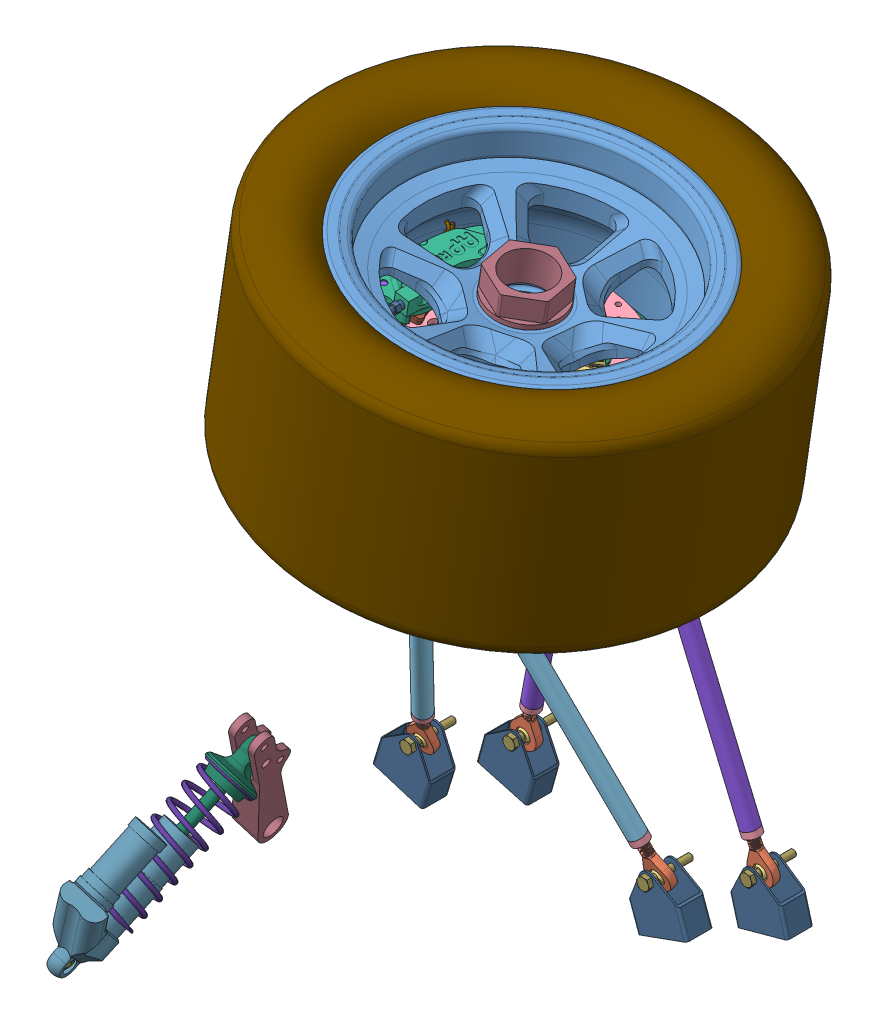
SolidWorks assembly WT-A0100-XA-Unsprung Front Axle Assembly, configuration Default. Lengths in mm.
Overall size (453.69 633.67 594.25).
81 component instances, 33 part files, 11 mates.
Components (placement in the parent):
- SP-A0200-AA-Upper Axle Assembly-1: SP-A0200-AA-Upper Axle Assembly [Default] at (-0.0001 -38.1 0) size (303.98 482.71 550.62)
  - Upper A-Arm^SP-A0200-AA-Upper Axle Assembly-1: Upper A-Arm^SP-A0200-AA-Upper Axle Assembly [Default] at (0 340.1778 -103.3743) x (1 0 0) z (0 -0.807933 0.589274) size (261.83 325.63 241.57) (virtual)
    - SP-Upper Apex Front-1: SP-Upper Apex Front [Default] at (789.6198 444.1063 49.8797) x (0.9592 -0.229397 0.165266) z (0 0.584537 0.811367) size (51.11 64.07 9.53)
    - MirrorFS-MALE ROD END UNF-3A, 0.3125x24-0.25D (XAM-4)1-1: MirrorFS-MALE ROD END UNF-3A, 0.3125x24-0.25D (XAM-4)1 [Default] at (912.4748 153.0246 259.5852) x (-0.946047 -0.262907 0.189408) z (0.32403 -0.767591 0.553) size (26.22 11.39 62.85)
      - MirrorBody^MirrorFS-MALE ROD END UNF-3A, 0.3125x24-0.25D (XAM-4)1-1: MirrorBody^MirrorFS-MALE ROD END UNF-3A, 0.3125x24-0.25D (XAM-4)1 [Default] at origin size (26.22 9.76 62.85) (virtual)
      - MirrorBall^MirrorFS-MALE ROD END UNF-3A, 0.3125x24-0.25D (XAM-4)1-1: MirrorBall^MirrorFS-MALE ROD END UNF-3A, 0.3125x24-0.25D (XAM-4)1 [Default] x (0.874091 -0.054164 -0.482733) z (-0.485762 -0.097546 -0.868631) size (12.7 9.53 12.7) (virtual)
    - MirrorFS-MALE ROD END UNF-3A, 0.3125x24-0.25D (XAM-4)1-2: MirrorFS-MALE ROD END UNF-3A, 0.3125x24-0.25D (XAM-4)1 [Default] at (683.8748 153.0246 259.5852) x (0.9592 -0.229397 0.165266) z (-0.28273 -0.778263 0.560688) size (26.22 11.39 62.85)
      - MirrorBody^MirrorFS-MALE ROD END UNF-3A, 0.3125x24-0.25D (XAM-4)1-1: MirrorBody^MirrorFS-MALE ROD END UNF-3A, 0.3125x24-0.25D (XAM-4)1 [Default] at origin size (26.22 9.76 62.85) (virtual)
      - MirrorBall^MirrorFS-MALE ROD END UNF-3A, 0.3125x24-0.25D (XAM-4)1-1: MirrorBall^MirrorFS-MALE ROD END UNF-3A, 0.3125x24-0.25D (XAM-4)1 [Default] x (0.874091 -0.054164 -0.482733) z (-0.485762 -0.097546 -0.868631) size (12.7 9.53 12.7) (virtual)
    - SP-10003-AB-Threaded Insert-1: SP-10003-AB-Threaded Insert [A-Arm] at (696.8946 188.8638 233.7654) x (-0.9592 0.229397 -0.165266) z (-0.28273 -0.778263 0.560688) size (15.88 15.88 15.88)
    - SP-10003-AB-Threaded Insert-2: SP-10003-AB-Threaded Insert [A-Arm] at (897.5532 188.3723 234.1194) x (0 0.584537 0.811367) z (0.32403 -0.767591 0.553) size (15.88 15.88 15.88)
    - SP-Upper A-Arm Tube-1: SP-Upper A-Arm Tube [Default] at (736.7473 298.5655 154.7324) x (0 -0.584537 -0.811367) z (0.9592 -0.229397 0.165266) size (15.88 313.5 15.88)
    - SP-Upper A-Arm Tube-2: SP-Upper A-Arm Tube [Default] at (851.8788 296.5698 156.1702) x (0 -0.584537 -0.811367) z (0.946047 0.262907 -0.189408) size (15.88 313.5 15.88)
    - FS-HIGH MISALIGN SPHERICAL BEARING, 0.375-0.906D (3072-6G)-1: FS-HIGH MISALIGN SPHERICAL BEARING, 0.375-0.906D (3072-6G) [Default] at (789.6198 444.1063 49.8797) x (-0.28273 -0.778263 0.560688) z (-0.9592 0.229397 -0.165266) size (26.46 21.71 26.13)
      - Race^FS-HIGH MISALIGN SPHERICAL BEARING, 0.375-0.906D (3072-6G)-1: Race^FS-HIGH MISALIGN SPHERICAL BEARING, 0.375-0.906D (3072-6G) [Default] at origin size (23.01 8.76 23.01) (virtual)
      - Ball^FS-HIGH MISALIGN SPHERICAL BEARING, 0.375-0.906D (3072-6G)-1: Ball^FS-HIGH MISALIGN SPHERICAL BEARING, 0.375-0.906D (3072-6G) [Default] x (0.359576 -0.008176 0.93308) z (-0.932238 -0.046516 0.358844) size (19.84 20.65 19.84) (virtual)
  - Lower A-Arm^SP-A0200-AA-Upper Axle Assembly-1: Lower A-Arm^SP-A0200-AA-Upper Axle Assembly [Default] at (0 -0.114 0.1797) x (1 0 0) z (0 0.000904 1) size (260.91 451.43 64.04) (virtual)
    - SP-Front Lower A-Arm Tube-2: SP-Front Lower A-Arm Tube [Default] at (852.4436 392.8879 96.9776) x (0.263467 -0.959286 -0.101763) z (0 -0.105491 0.99442) size (374.92 15.88 15.88)
    - MirrorFS-MALE ROD END UNF-3A, 0.3125x24-0.25D (XAM-4)1-1: MirrorFS-MALE ROD END UNF-3A, 0.3125x24-0.25D (XAM-4)1 [Default] at (912.4748 174.3139 73.7908) x (0.964668 0.261997 0.027793) z (0.263467 -0.959286 -0.101763) size (26.22 11.39 62.85)
      - MirrorBody^MirrorFS-MALE ROD END UNF-3A, 0.3125x24-0.25D (XAM-4)1-1: MirrorBody^MirrorFS-MALE ROD END UNF-3A, 0.3125x24-0.25D (XAM-4)1 [Default] at origin size (26.22 9.76 62.85) (virtual)
      - MirrorBall^MirrorFS-MALE ROD END UNF-3A, 0.3125x24-0.25D (XAM-4)1-1: MirrorBall^MirrorFS-MALE ROD END UNF-3A, 0.3125x24-0.25D (XAM-4)1 [Default] x (0.874091 -0.054164 -0.482733) z (-0.485762 -0.097546 -0.868631) size (12.7 9.53 12.7) (virtual)
    - MirrorFS-MALE ROD END UNF-3A, 0.3125x24-0.25D (XAM-4)1-2: MirrorFS-MALE ROD END UNF-3A, 0.3125x24-0.25D (XAM-4)1 [Default] at (683.8748 174.3139 73.7908) x (0.964668 -0.261997 -0.027793) z (-0.263467 -0.959286 -0.101763) size (26.22 11.39 62.85)
      - MirrorBody^MirrorFS-MALE ROD END UNF-3A, 0.3125x24-0.25D (XAM-4)1-1: MirrorBody^MirrorFS-MALE ROD END UNF-3A, 0.3125x24-0.25D (XAM-4)1 [Default] at origin size (26.22 9.76 62.85) (virtual)
      - MirrorBall^MirrorFS-MALE ROD END UNF-3A, 0.3125x24-0.25D (XAM-4)1-1: MirrorBall^MirrorFS-MALE ROD END UNF-3A, 0.3125x24-0.25D (XAM-4)1 [Default] x (0.874091 -0.054164 -0.482733) z (-0.485762 -0.097546 -0.868631) size (12.7 9.53 12.7) (virtual)
    - SP-Lower Apex Front-1: SP-Lower Apex Front [Default] at (798.1748 590.481 117.9388) x (0.964668 -0.261997 -0.027793) z (0 -0.105491 0.99442) size (48.15 64.07 9.53)
    - SP-10003-AB-Threaded Insert-1: SP-10003-AB-Threaded Insert [A-Arm] at (900.7637 216.9541 78.3142) x (0.964668 0.261997 0.027793) z (0.263467 -0.959286 -0.101763) size (15.88 15.88 15.88)
    - SP-10003-AB-Threaded Insert-2: SP-10003-AB-Threaded Insert [A-Arm] at (695.5859 216.9541 78.3142) x (0.964668 -0.261997 -0.027793) z (-0.263467 -0.959286 -0.101763) size (15.88 15.88 15.88)
    - FS-HIGH MISALIGN SPHERICAL BEARING, 0.375-0.906D (3072-6G)-1: FS-HIGH MISALIGN SPHERICAL BEARING, 0.375-0.906D (3072-6G) [Default] at (798.1748 590.481 117.9388) x (0.263467 0.959286 0.101763) z (-0.964668 0.261997 0.027793) size (26.46 21.71 26.13)
      - Race^FS-HIGH MISALIGN SPHERICAL BEARING, 0.375-0.906D (3072-6G)-1: Race^FS-HIGH MISALIGN SPHERICAL BEARING, 0.375-0.906D (3072-6G) [Default] at origin size (23.01 8.76 23.01) (virtual)
      - Ball^FS-HIGH MISALIGN SPHERICAL BEARING, 0.375-0.906D (3072-6G)-1: Ball^FS-HIGH MISALIGN SPHERICAL BEARING, 0.375-0.906D (3072-6G) [Default] x (0.359576 -0.008176 0.93308) z (-0.932238 -0.046516 0.358844) size (19.84 20.65 19.84) (virtual)
    - SP-Front Lower A-Arm Tube-3: SP-Front Lower A-Arm Tube [Default] at (743.906 392.8879 96.9776) x (-0.263467 -0.959286 -0.101763) z (0 -0.105491 0.99442) size (374.92 15.88 15.88)
  - SP-C30066-AA-A-Arm Tab Box-2: SP-C30066-AA-A-Arm Tab Box [Default] at (918.3945 204.1953 173.2262) x (-0.338991 0.94079 0) z (-0.94079 -0.338991 0) size (50.8 25.4 50.8)
  - SP-C30066-AA-A-Arm Tab Box-3: SP-C30066-AA-A-Arm Tab Box [Default] at (678.702 203.9451 173.2262) x (0.296224 0.955119 0) z (-0.955119 0.296224 0) size (50.8 25.4 50.8)
  - SP-C30066-AA-A-Arm Tab Box-4: SP-C30066-AA-A-Arm Tab Box [Default] at (917.0992 157.4275 73.8128) x (-0.264819 0.964298 0) z (-0.964298 -0.264819 0) size (50.8 25.4 50.8)
  - SP-C30066-AA-A-Arm Tab Box-5: SP-C30066-AA-A-Arm Tab Box [Default] at (679.2504 157.4275 73.8128) x (0.264819 0.964298 0) z (-0.964298 0.264819 0) size (50.8 25.4 50.8)
  - MirrorSP-30063-AB-Pushrod Tab-1: MirrorSP-30063-AB-Pushrod Tab [Default] at (810.0811 564.8807 118.0854) x (1 0 0) z (0 0.104591 -0.994515) size (1.59 15.88 23.81)
  - MirrorSP-30063-AB-Pushrod Tab-2: MirrorSP-30063-AB-Pushrod Tab [Default] at (786.2686 564.8807 118.0854) x (1 0 0) z (0 0.104591 -0.994515) size (1.59 15.88 23.81)
  - FS-CADMIUM PLATED C3 HEX, 0.25x28-1.65-0.469 (AN4-13A)-1: FS-CADMIUM PLATED C3 HEX, 0.25x28-1.65-0.469 (AN4-13A) [Default] at (912.4748 220.6238 167.1556) x (0 0 -1) z (0.923728 0.383049 0) size (46.28 12.9 11.18)
  - FS-CADMIUM PLATED C3 HEX, 0.25x28-1.65-0.469 (AN4-13A)-2: FS-CADMIUM PLATED C3 HEX, 0.25x28-1.65-0.469 (AN4-13A) [Default] at (683.8748 220.6238 167.1556) x (0 0 -1) z (-0.703898 0.710301 0) size (46.28 12.9 11.18)
  - FS-CADMIUM PLATED C3 HEX, 0.25x28-1.65-0.469 (AN4-13A)-3: FS-CADMIUM PLATED C3 HEX, 0.25x28-1.65-0.469 (AN4-13A) [Default] at (683.8748 174.2666 67.7422) x (0 0 -1) z (0.923728 0.383049 0) size (46.28 12.9 11.18)
  - FS-CADMIUM PLATED C3 HEX, 0.25x28-1.65-0.469 (AN4-13A)-4: FS-CADMIUM PLATED C3 HEX, 0.25x28-1.65-0.469 (AN4-13A) [Default] at (912.4748 174.2666 67.7422) x (0 0 -1) z (0.923728 0.383049 0) size (46.28 12.9 11.18)
  - FS-CADMIUM PLATED C3 HEX, 0.25x28-1.65-0.469 (AN4-13A)-5: FS-CADMIUM PLATED C3 HEX, 0.25x28-1.65-0.469 (AN4-13A) [Default] at (792.898 563.2203 133.8733) x (-1 0 0) z (0 0.932323 -0.361628) size (46.28 12.9 11.18)
  - SP-Front Rocker-1: SP-Front Rocker [Default] at (695.7947 245.9593 342.2966) x (0.944914 -0.325775 -0.03174) z (-0.096211 -0.369123 0.924387) size (25.4 150.81 36.51)
  - SP-A0105-AC-Ohlin TTX25 MKII, 200mm-2: SP-A0105-AC-Ohlin TTX25 MKII, 200mm [Default] at (691.0804 214.2429 527.4807) x (0.944914 -0.325775 -0.03174) z (-0.189123 -0.622541 0.759392) size (48.39 85.02 216)
    - Shock Body^SP-A0105-AC-Ohlin TTX25 MKII, 200mm-1: Shock Body^SP-A0105-AC-Ohlin TTX25 MKII, 200mm [Default] at origin size (40.76 80 131.7) (virtual)
    - Head^SP-A0105-AC-Ohlin TTX25 MKII, 200mm-1: Head^SP-A0105-AC-Ohlin TTX25 MKII, 200mm [Default] at (0 0 -193) size (46 46 119) (virtual)
    - Ball^SP-A0105-AC-Ohlin TTX25 MKII, 200mm-1: Ball^SP-A0105-AC-Ohlin TTX25 MKII, 200mm [Default] at (0 0 -193) x (-0.011681 0.107343 0.994153) z (0.993776 0.111394 -0.000351) size (15 15 8) (virtual)
    - Ball^SP-A0105-AC-Ohlin TTX25 MKII, 200mm-2: Ball^SP-A0105-AC-Ohlin TTX25 MKII, 200mm [Default] x (0.079523 -0.862756 -0.499328) z (0.965926 -0.057074 0.252448) size (15 15 8) (virtual)
    - SP-#####-AB-Spring-1: SP-#####-AB-Spring [Default] at (0 0 -169.5) size (48.39 49.05 127.97)
- WT-A0100-AC-Corner Assembly-1: WT-A0100-AC-Corner Assembly [Front Left Corner Assembly] at (800.0242 576.744 198.2101) x (0.98768 -0.153849 -0.028614) z (0.030919 0.012613 0.999442) size (411.48 224.2 416.93)
  - WT-00202-AA-Hoosier R25B 16x7_5-10-1: WT-00202-AA-Hoosier R25B 16x7_5-10 [Default] x (1 0 0) z (0 -0.999657 -0.026177) size (411.48 411.48 213.5)
  - WT-00201-AA-OZ Centerlock 10in Wheel-1: WT-00201-AA-OZ Centerlock 10in Wheel [Default] at (0 21.9925 0.5759) x (0.796774 -0.015818 0.60407) z (0 0.999657 0.026177) size (288.79 288.79 189.86)
  - WT-10105-AA-Drive Pin-8: WT-10105-AA-Drive Pin [Default] at (-24.1711 21.1582 32.4359) x (0.363068 -0.024391 0.931443) z (-0.931762 -0.009504 0.362944) size (12.67 23.01 11.95)
  - BR-20602-AB-Brake Hat-2: BR-20602-AB-Brake Hat [Default] at (0 -4.1288 -0.1081) x (-0.921706 -0.010154 0.387755) z (-0.387888 0.024127 -0.921391) size (120.29 4.76 113.7)
  - BR-20601-AA-Brake Rotor-1: BR-20601-AA-Brake Rotor [Default] at (0 -4.1288 -0.1081) x (-0.796774 0.015818 -0.60407) z (0.604277 0.020857 -0.796501) size (190.5 4.76 190.5)
  - CP4227-2S0-1: CP4227-2S0 [Default] at (15.875 -4.1288 -0.1081) x (0.99863 -0.00137 0.052318) z (-0.052336 -0.026141 0.998287) size (71.54 66.42 130.94)
    - CP4227-2S0.STEP-1: CP4227-2S0.STEP [Default] x (0 0 -1) z (0 -1 0) size (130.94 71.54 66.42)
      - CP4227-101.STEP-1: CP4227-101.STEP [Default] at origin size (112 60.5 34.68)
      - CP4227-102.STEP-1: CP4227-102.STEP [Default] x (-1 0 0) z (0 0 -1) size (109 47.57 30.98)
      - cp3049-40a_CP4226-103.STEP-1: cp3049-40a_CP4226-103.STEP [Default] at (-23.4668 -94.12 -10.305) size (25.2 25.2 14.87)
      - cp3049-40a_CP4226-103.STEP-2: cp3049-40a_CP4226-103.STEP [Default] at (-23.4668 -94.12 10.305) x (-0.98369 0.179874 0) z (0 0 -1) size (25.2 25.2 14.87)
      - cp3049-40a_CP4226-103.STEP-3: cp3049-40a_CP4226-103.STEP [Default] at (23.4668 -94.12 10.305) x (-0.960147 0.279495 0) z (0 0 -1) size (25.2 25.2 14.87)
      - cp3049-40a_CP4226-103.STEP-4: cp3049-40a_CP4226-103.STEP [Default] at (23.4668 -94.12 -10.305) size (25.2 25.2 14.87)
      - cp3838-M08x1.25m_CP4477-110.STEP-1: cp3838-M08x1.25m_CP4477-110.STEP [Default] at (-41.1 -109.6 19.55) x (-0.998897 0.046962 0) z (0 0 -1) size (13 13 46)
      - cp3838-M08x1.25m_CP4477-110.STEP-2: cp3838-M08x1.25m_CP4477-110.STEP [Default] at (0 -116.83 19.55) x (-0.99038 0.138378 0) z (0 0 -1) size (13 13 46)
      - cp3838-M08x1.25m_CP4477-110.STEP-3: cp3838-M08x1.25m_CP4477-110.STEP [Default] at (41.1 -109.6 19.55) x (-1 -0.000032 0) z (0 0 -1) size (13 13 46)
      - cp4226-104_CP4226-104.STEP-1: cp4226-104_CP4226-104.STEP [Default] at (-29.0318 -116.44 -31.75) x (0 0 1) z (1 0 0) size (61.35 20.1 3)
      - cp4226-104_CP4226-104.STEP-2: cp4226-104_CP4226-104.STEP [Default] at (29.0318 -116.44 -31.75) x (0 0 1) z (1 0 0) size (61.35 20.1 3)
      - CP4469-101.STEP-1: CP4469-101.STEP [Default] at (-65.47 -82.62 -23.98) x (0 0.474307 -0.88036) z (1 0 0) size (9.24 8.21 29.15)
      - CP4469-101.STEP-2: CP4469-101.STEP [Default] at (65.47 -82.62 -23.98) x (0 0.509894 0.860237) z (-1 0 0) size (9.24 8.21 29.15)
      - CP4226-4m.STEP-1: CP4226-4m.STEP [Default] at (10.0433 -40.2815 10.305) x (0.970296 0.241922 0) z (0 0 -1) size (39.7 43.64 7)
      - CP4226-4m.STEP-2: CP4226-4m.STEP [Default] at (10.0433 -40.2815 -10.305) x (-0.970296 -0.241922 0) z (0 0 1) size (39.7 43.64 7)
      - CP4226-4m.STEP-3: CP4226-4m.STEP [Default] at (-10.0433 -40.2815 -10.305) x (-0.970296 0.241922 0) z (0 0 1) size (39.7 43.64 7)
      - CP4226-4m.STEP-4: CP4226-4m.STEP [Default] at (-10.0433 -40.2815 10.305) x (0.970296 -0.241922 0) z (0 0 -1) size (39.7 43.64 7)
  - WT-20104-AB-Sensor Ring-1: WT-20104-AB-Sensor Ring [Default] at (0 -6.5093 -0.1705) x (-0.796774 0.015818 -0.60407) z (0 -0.999657 -0.026177) size (121.12 121.92 1.59)
  - WT-10105-AA-Drive Pin-18: WT-10105-AA-Drive Pin [Default] at (-31.871 22.6252 -23.5869) x (-0.931762 -0.009504 0.362944) z (-0.363068 0.024391 -0.931443) size (12.67 23.01 11.95)
  - WT-10105-AA-Drive Pin-19: WT-10105-AA-Drive Pin [Default] at (24.1711 22.8267 -31.2842) x (-0.363068 0.024391 -0.931443) z (0.931762 0.009504 -0.362944) size (12.67 23.01 11.95)
  - WT-10105-AA-Drive Pin-20: WT-10105-AA-Drive Pin [Default] at (31.871 21.3597 24.7387) x (0.931762 0.009504 -0.362944) z (0.363068 -0.024391 0.931443) size (12.67 23.01 11.95)
  - WT-10102-AA-Centerlock Nut-1: WT-10102-AA-Centerlock Nut [Default] at (0 72.5945 1.901) x (-0.92317 0.010062 -0.38426) z (0.384391 0.024166 -0.922854) size (66 31.75 66)
  - WT-AA-Camber Block-1: WT-AA-Camber Block [Default] at (-4.553 -27.8797 86.1755) x (-0.99863 0.00137 -0.052318) z (-0.052336 -0.026141 0.998287) size (47.63 44.45 33.35)
  - WT-AC-Upright-1: WT-AC-Upright [Default] at (0 -38.7684 -1.0152) x (-0.99863 0.00137 -0.052318) z (-0.052336 -0.026141 0.998287) size (124.72 50.63 207.18)
Mates (geometry in assembly coordinates):
- Distance1: distance = 912.4747 mm: point of SP-A0200-AA-Upper Axle Assembly-1/Upper A-Arm^SP-A0200-AA-Upper Axle Assembly-1; plane of assembly
- Distance2: distance = 683.8747 mm: point of SP-A0200-AA-Upper Axle Assembly-1/Upper A-Arm^SP-A0200-AA-Upper Axle Assembly-1; plane of assembly
- Distance3: distance = 182.5238 mm: point of SP-A0200-AA-Upper Axle Assembly-1/Upper A-Arm^SP-A0200-AA-Upper Axle Assembly-1; plane of assembly
- Distance4: distance = 182.5238 mm: point of SP-A0200-AA-Upper Axle Assembly-1/Upper A-Arm^SP-A0200-AA-Upper Axle Assembly-1; plane of assembly
- Distance5: distance = 173.2262 mm: point of SP-A0200-AA-Upper Axle Assembly-1/Upper A-Arm^SP-A0200-AA-Upper Axle Assembly-1; plane of assembly
- Distance6: distance = 73.8128 mm: point of SP-A0200-AA-Upper Axle Assembly-1/Lower A-Arm^SP-A0200-AA-Upper Axle Assembly-1; plane of assembly
- Distance7: distance = 284.8254 mm: point of WT-A0100-AC-Corner Assembly-1; plane of assembly
- Distance8: distance = 561.5788 mm: plane of assembly; point of WT-A0100-AC-Corner Assembly-1; plane of SP-A0200-AA-Upper Axle Assembly-1 through (-0.0001 -38.1 0) normal (0 1 0)
- Distance9: distance = 789.62 mm: point of WT-A0100-AC-Corner Assembly-1; plane of assembly
- Distance11: distance = 590.4738 mm: plane of assembly; point of WT-A0100-AC-Corner Assembly-1; plane of SP-A0200-AA-Upper Axle Assembly-1 through (-0.0001 -38.1 0) normal (0 1 0)
- Distance12: distance = 798.1747 mm: plane of assembly; point of WT-A0100-AC-Corner Assembly-1; plane of SP-A0200-AA-Upper Axle Assembly-1 through (-0.0001 -38.1 0) normal (1 0 0)
